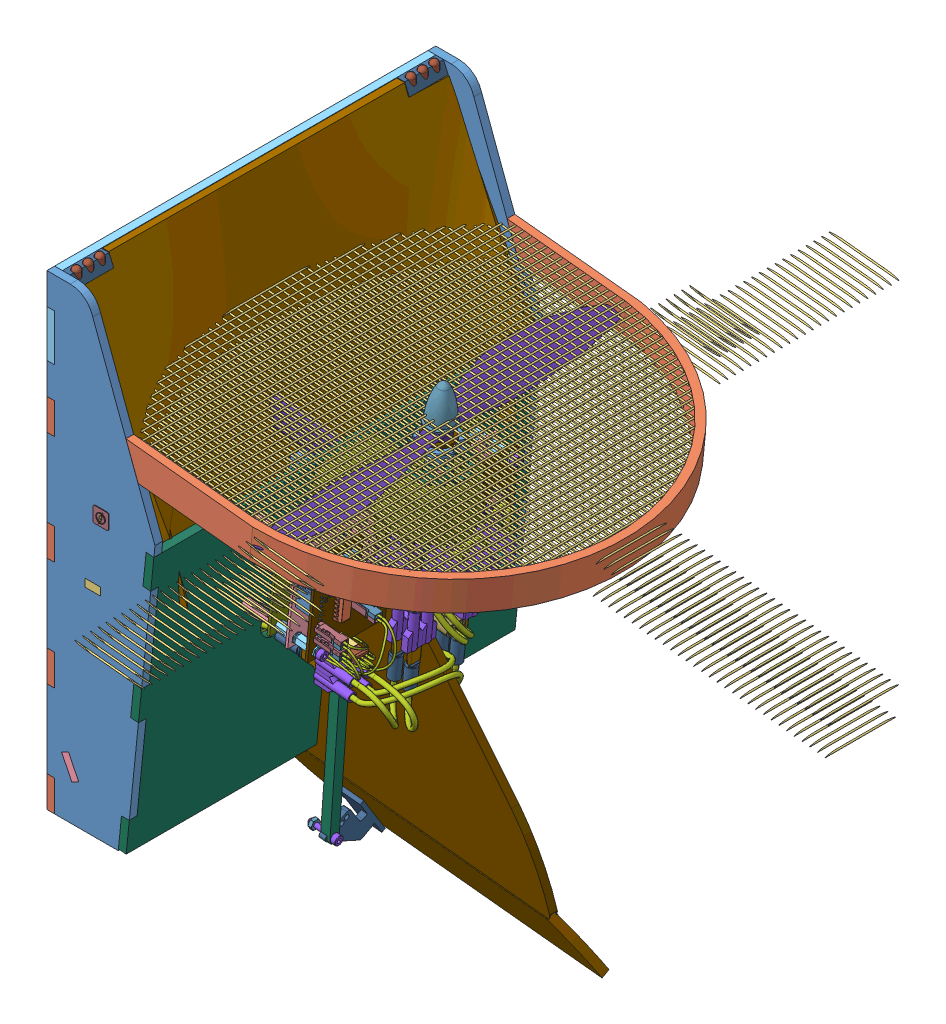
SolidWorks assembly AssTotaleSimu, configuration Défaut. Lengths in mm. (continued)
Components (placement in the parent): (continued)
- AssStructSimu-1: AssStructSimu [Défaut] at (-125.7658 -1.8483 624.6548) x (1 0 0) z (0 0 -1) size (323.53 326.04 251.6) (continued)
  - AssCarte-1: AssCarte [Défaut] at (-42.8534 32.2132 302.028) x (-0.101852 0.9948 0) z (0.9948 0.101852 0) size (91.19 130.57 98.45) (continued)
    - carte_onduleur_v4-1: carte_onduleur_v4 [Défaut] at (-25.7639 0.8332 112.9379) size (66.52 130.57 82.34) (continued)
      - CARTE_CMD-1: CARTE_CMD [Défaut] at (25 57.2 0.803) size (60.1 130 26.71) (continued)
        - Open CASCADE STEP translator 6.8 1.20.1-1: Open CASCADE STEP translator 6.8 1.20.1 [Défaut] at origin size (60.1 130 26.71) (continued)
          - Body_1_4-1: Body_1_4 [Défaut] at (-55 5 12) size (60.1 130 26.71) (continued)
            - 40_2-1: 40_2 [Défaut] at (26.2 -12.2 0.803) x (0 -1 0) z (0 0 1) size (2.34 1.04 0.5) (continued)
              - =_[0_1_1_30]-1: =_[0_1_1_30] [Défaut] at origin size (2.34 1.04 0.5) (continued)
                - 33_2-1: 33_2 [Défaut] at (0.3048 0 0) x (-1 0 0) z (0 0 1) size (0.51 1.02 0.5)
                - 34-1: 34 [Défaut] at origin size (0.51 1.02 0.5)
            - 42_2-1: 42_2 [Défaut] at (24.4 -119.2 0.803) size (2.34 1.04 0.5)
              - =_[0_1_1_30]-1: =_[0_1_1_30] [Défaut] at origin size (2.34 1.04 0.5)
                - 32_2-1: 32_2 [Défaut] at origin size (2.29 1.04 0.43)
                - 33_2-1: 33_2 [Défaut] at (0.3048 0 0) x (-1 0 0) z (0 0 1) size (0.51 1.02 0.5)
                - 34-1: 34 [Défaut] at origin size (0.51 1.02 0.5)
            - 45-1: 45 [Défaut] at (46.4 -125 0.803) size (5.08 5 14.3)
              - =_[0_1_1_38]-1: =_[0_1_1_38] [Défaut] at origin size (5.08 5 14.3)
                - 190-1: 190 [Défaut] at (1.2 0 11) size (5.08 5 14.3)
            - 48-1: 48 [Défaut] at (40.1 -125 0.803) size (5.08 5 14.3)
              - =_[0_1_1_41]-1: =_[0_1_1_41] [Défaut] at origin size (5.08 5 14.3)
                - 190-1: 190 [Défaut] at (1.2 0 11) size (5.08 5 14.3)
            - 51-1: 51 [Défaut] at (6.4 -119.9 0.803) x (0 1 0) z (0 0 1) size (15.24 2.54 7.37)
              - =_[0_1_1_43]-1: =_[0_1_1_43] [Défaut] at origin size (15.24 2.54 7.37)
                - 49_2-1: 49_2 [Défaut] at (6.5 0 0) x (1 0 0) z (0 -1 0) size (15.24 7.37 2.54)
            - 57_2-1: 57_2 [Défaut] at (50.8796 -121.1 -0.803) x (-1 0 0) z (0 0 -1) size (2.54 1.98 0.64)
              - =_[0_1_1_46]-1: =_[0_1_1_46] [Défaut] at origin size (2.54 1.98 0.64)
                - 52-1: 52 [Défaut] at origin size (2.54 1.14 0.58)
                - 53-1: 53 [Défaut] x (0 -1 0) z (0 0 1) size (0.43 0.51 0.38)
                - 54-1: 54 [Défaut] at (1.8796 1.8796 0) x (0 -1 0) z (0 0 1) size (0.43 0.51 0.38)
                - 55-1: 55 [Défaut] at (-0.9652 -2.8448 0) x (0 1 0) z (0 0 1) size (0.41 0.51 0.38)
            - 59_2-1: 59_2 [Défaut] at (43.6398 -120.995 -0.803) x (-1 0 0) z (0 0 -1) size (2.54 1.98 0.64)
              - =_[0_1_1_46]-1: =_[0_1_1_46] [Défaut] at origin size (2.54 1.98 0.64)
                - 52-1: 52 [Défaut] at origin size (2.54 1.14 0.58)
                - 53-1: 53 [Défaut] x (0 -1 0) z (0 0 1) size (0.43 0.51 0.38)
                - 54-1: 54 [Défaut] at (1.8796 1.8796 0) x (0 -1 0) z (0 0 1) size (0.43 0.51 0.38)
                - 55-1: 55 [Défaut] at (-0.9652 -2.8448 0) x (0 1 0) z (0 0 1) size (0.41 0.51 0.38)
            - 61_2-1: 61_2 [Défaut] at (47.6 -119.9 -0.803) x (-1 0 0) z (0 0 -1) size (2.34 1.04 0.5)
              - =_[0_1_1_30]-1: =_[0_1_1_30] [Défaut] at origin size (2.34 1.04 0.5)
                - 32_2-1: 32_2 [Défaut] at origin size (2.29 1.04 0.43)
                - 33_2-1: 33_2 [Défaut] at (0.3048 0 0) x (-1 0 0) z (0 0 1) size (0.51 1.02 0.5)
                - 34-1: 34 [Défaut] at origin size (0.51 1.02 0.5)
            - 63-1: 63 [Défaut] at (40.4 -119.9 -0.803) x (-1 0 0) z (0 0 -1) size (2.34 1.04 0.5)
              - =_[0_1_1_30]-1: =_[0_1_1_30] [Défaut] at origin size (2.34 1.04 0.5)
                - 32_2-1: 32_2 [Défaut] at origin size (2.29 1.04 0.43)
                - 33_2-1: 33_2 [Défaut] at (0.3048 0 0) x (-1 0 0) z (0 0 1) size (0.51 1.02 0.5)
                - 34-1: 34 [Défaut] at origin size (0.51 1.02 0.5)
            - 68-1: 68 [Défaut] at (47.7 -21.8 -0.803) x (0 1 0) z (0 0 -1) size (2.34 1.04 0.5)
              - =_[0_1_1_55]-1: =_[0_1_1_55] [Défaut] at origin size (2.34 1.04 0.5)
                - 64-1: 64 [Défaut] at origin size (2.29 1.04 0.43)
                - 65-1: 65 [Défaut] at (0.3048 0 0) x (-1 0 0) z (0 0 1) size (0.51 1.02 0.5)
                - 66-1: 66 [Défaut] at origin size (0.51 1.02 0.5)
            - 70-1: 70 [Défaut] at (47.6 -121.7 -0.803) x (-1 0 0) z (0 0 -1) size (2.34 1.04 0.5)
              - =_[0_1_1_30]-1: =_[0_1_1_30] [Défaut] at origin size (2.34 1.04 0.5)
                - 32_2-1: 32_2 [Défaut] at origin size (2.29 1.04 0.43)
                - 33_2-1: 33_2 [Défaut] at (0.3048 0 0) x (-1 0 0) z (0 0 1) size (0.51 1.02 0.5)
                - 34-1: 34 [Défaut] at origin size (0.51 1.02 0.5)
            - 72-1: 72 [Défaut] at (40.4 -121.5 -0.803) x (-1 0 0) z (0 0 -1) size (2.34 1.04 0.5)
              - =_[0_1_1_30]-1: =_[0_1_1_30] [Défaut] at origin size (2.34 1.04 0.5)
                - 32_2-1: 32_2 [Défaut] at origin size (2.29 1.04 0.43)
                - 33_2-1: 33_2 [Défaut] at (0.3048 0 0) x (-1 0 0) z (0 0 1) size (0.51 1.02 0.5)
                - 34-1: 34 [Défaut] at origin size (0.51 1.02 0.5)
            - 74-1: 74 [Défaut] at (47.7 -18.3 -0.803) x (0 1 0) z (0 0 -1) size (2.34 1.04 0.5)
              - =_[0_1_1_55]-1: =_[0_1_1_55] [Défaut] at origin size (2.34 1.04 0.5)
                - 64-1: 64 [Défaut] at origin size (2.29 1.04 0.43)
                - 65-1: 65 [Défaut] at (0.3048 0 0) x (-1 0 0) z (0 0 1) size (0.51 1.02 0.5)
                - 66-1: 66 [Défaut] at origin size (0.51 1.02 0.5)
            - 76-1: 76 [Défaut] at (45.5 -118.3 -0.803) x (1 0 0) z (0 0 -1) size (2.34 1.04 0.5)
              - =_[0_1_1_30]-1: =_[0_1_1_30] [Défaut] at origin size (2.34 1.04 0.5)
                - 32_2-1: 32_2 [Défaut] at origin size (2.29 1.04 0.43)
                - 33_2-1: 33_2 [Défaut] at (0.3048 0 0) x (-1 0 0) z (0 0 1) size (0.51 1.02 0.5)
                - 34-1: 34 [Défaut] at origin size (0.51 1.02 0.5)
            - 78-1: 78 [Défaut] at (38.2 -118.3 -0.803) x (1 0 0) z (0 0 -1) size (2.34 1.04 0.5)
              - =_[0_1_1_30]-1: =_[0_1_1_30] [Défaut] at origin size (2.34 1.04 0.5)
                - 32_2-1: 32_2 [Défaut] at origin size (2.29 1.04 0.43)
                - 33_2-1: 33_2 [Défaut] at (0.3048 0 0) x (-1 0 0) z (0 0 1) size (0.51 1.02 0.5)
                - 34-1: 34 [Défaut] at origin size (0.51 1.02 0.5)
            - 80-1: 80 [Défaut] at (28.6 -10.7 0.803) x (0 1 0) z (0 0 1) size (2.34 1.04 0.5)
              - =_[0_1_1_55]-1: =_[0_1_1_55] [Défaut] at origin size (2.34 1.04 0.5)
                - 64-1: 64 [Défaut] at origin size (2.29 1.04 0.43)
                - 65-1: 65 [Défaut] at (0.3048 0 0) x (-1 0 0) z (0 0 1) size (0.51 1.02 0.5)
                - 66-1: 66 [Défaut] at origin size (0.51 1.02 0.5)
            - 82-1: 82 [Défaut] at (23.7 -10.7 0.803) x (0 1 0) z (0 0 1) size (2.34 1.04 0.5)
              - =_[0_1_1_55]-1: =_[0_1_1_55] [Défaut] at origin size (2.34 1.04 0.5)
                - 64-1: 64 [Défaut] at origin size (2.29 1.04 0.43)
                - 65-1: 65 [Défaut] at (0.3048 0 0) x (-1 0 0) z (0 0 1) size (0.51 1.02 0.5)
                - 66-1: 66 [Défaut] at origin size (0.51 1.02 0.5)
            - 84-1: 84 [Défaut] at (26.2 -10.7 0.803) x (0 1 0) z (0 0 1) size (2.34 1.04 0.5)
              - =_[0_1_1_55]-1: =_[0_1_1_55] [Défaut] at origin size (2.34 1.04 0.5)
                - 64-1: 64 [Défaut] at origin size (2.29 1.04 0.43)
                - 65-1: 65 [Défaut] at (0.3048 0 0) x (-1 0 0) z (0 0 1) size (0.51 1.02 0.5)
                - 66-1: 66 [Défaut] at origin size (0.51 1.02 0.5)
            - 86-1: 86 [Défaut] at (23.0336 -119.2 0.803) x (-1 0 0) z (0 0 1) size (2.34 1.04 0.5)
              - =_[0_1_1_55]-1: =_[0_1_1_55] [Défaut] at origin size (2.34 1.04 0.5)
                - 64-1: 64 [Défaut] at origin size (2.29 1.04 0.43)
                - 65-1: 65 [Défaut] at (0.3048 0 0) x (-1 0 0) z (0 0 1) size (0.51 1.02 0.5)
                - 66-1: 66 [Défaut] at origin size (0.51 1.02 0.5)
            - 88-1: 88 [Défaut] at (14.1 -114.2 0.803) x (0 -1 0) z (0 0 1) size (2.34 1.04 0.5)
              - =_[0_1_1_55]-1: =_[0_1_1_55] [Défaut] at origin size (2.34 1.04 0.5)
                - 64-1: 64 [Défaut] at origin size (2.29 1.04 0.43)
                - 65-1: 65 [Défaut] at (0.3048 0 0) x (-1 0 0) z (0 0 1) size (0.51 1.02 0.5)
                - 66-1: 66 [Défaut] at origin size (0.51 1.02 0.5)
            - 90-1: 90 [Défaut] at (43.6 -107.8 -0.803) x (1 0 0) z (0 0 -1) size (2.34 1.04 0.5)
              - =_[0_1_1_55]-1: =_[0_1_1_55] [Défaut] at origin size (2.34 1.04 0.5)
                - 64-1: 64 [Défaut] at origin size (2.29 1.04 0.43)
                - 65-1: 65 [Défaut] at (0.3048 0 0) x (-1 0 0) z (0 0 1) size (0.51 1.02 0.5)
                - 66-1: 66 [Défaut] at origin size (0.51 1.02 0.5)
            - 92-1: 92 [Défaut] at (43.6 -106 -0.803) x (1 0 0) z (0 0 -1) size (2.34 1.04 0.5)
              - =_[0_1_1_55]-1: =_[0_1_1_55] [Défaut] at origin size (2.34 1.04 0.5)
                - 64-1: 64 [Défaut] at origin size (2.29 1.04 0.43)
                - 65-1: 65 [Défaut] at (0.3048 0 0) x (-1 0 0) z (0 0 1) size (0.51 1.02 0.5)
                - 66-1: 66 [Défaut] at origin size (0.51 1.02 0.5)
            - 175-1: 175 [Défaut] at (10 -21.7 0.803) x (0 -1 0) z (0 0 1) size (15 25.4 12.78)
              - =_[0_1_1_72]-1: =_[0_1_1_72] [Défaut] at origin size (15 25.4 12.78)
                - 173-1: 173 [Défaut] at (-1.4 -1 12) x (-1 0 0) z (0 1 0) size (15 12.78 25.4)
                  - board_1-1: board_1 [Défaut] at (-7.5 -1.57 12.5) size (15 1.57 25)
                  - hole_plating_20-1: hole_plating_20 [Défaut] at (-1.5 0 23.93) size (1.5 0.01 1.5)
                  - hole_plating_20-2: hole_plating_20 [Défaut] at (-1.5 0 21.39) size (1.5 0.01 1.5)
                  - hole_plating_20-3: hole_plating_20 [Défaut] at (-1.5 0 8.69) size (1.5 0.01 1.5)
                  - hole_plating_20-4: hole_plating_20 [Défaut] at (-1.5 -1.58 13.77) size (1.5 0.01 1.5)
                  - hole_plating_20-5: hole_plating_20 [Défaut] at (-1.5 0 16.31) size (1.5 0.01 1.5)
                  - hole_plating_20-6: hole_plating_20 [Défaut] at (-1.5 0 18.85) size (1.5 0.01 1.5)
                  - hole_plating_20-7: hole_plating_20 [Défaut] at (-1.5 0 13.77) size (1.5 0.01 1.5)
                  - hole_plating_20-8: hole_plating_20 [Défaut] at (-1.5 -1.58 11.23) size (1.5 0.01 1.5)
                  - hole_plating_20-9: hole_plating_20 [Défaut] at (-1.5 -1.58 18.85) size (1.5 0.01 1.5)
                  - hole_plating_20-10: hole_plating_20 [Défaut] at (-1.5 -1.58 6.15) size (1.5 0.01 1.5)
                  - hole_plating_20-11: hole_plating_20 [Défaut] at (-1.5 0 1.07) size (1.5 0.01 1.5)
                  - hole_plating_20-12: hole_plating_20 [Défaut] at (-1.5 -1.58 3.61) size (1.5 0.01 1.5)
                  - hole_plating_20-13: hole_plating_20 [Défaut] at (-1.5 -1.58 1.07) size (1.5 0.01 1.5)
                  - hole_plating_20-14: hole_plating_20 [Défaut] at (-1.5 -1.58 8.69) size (1.5 0.01 1.5)
                  - hole_plating_20-15: hole_plating_20 [Défaut] at (-1.5 -1.58 16.31) size (1.5 0.01 1.5)
                  - hole_plating_20-16: hole_plating_20 [Défaut] at (-1.5 0 11.23) size (1.5 0.01 1.5)
                  - hole_plating_20-17: hole_plating_20 [Défaut] at (-1.5 0 3.61) size (1.5 0.01 1.5)
                  - hole_plating_20-18: hole_plating_20 [Défaut] at (-1.5 -1.58 21.39) size (1.5 0.01 1.5)
                  - hole_plating_20-19: hole_plating_20 [Défaut] at (-1.5 0 6.15) size (1.5 0.01 1.5)
                  - hole_plating_20-20: hole_plating_20 [Défaut] at (-1.5 -1.58 23.93) size (1.5 0.01 1.5)
                  - Pin_Header_1x10_TH_Pitch_2.54mm_1-1: Pin_Header_1x10_TH_Pitch_2.54mm_1 [Défaut] at (-1.5 -1.5786 23.93) x (0 0 -1) z (0 -1 0) size (25.4 2.54 12.7)
                    - 124-1: 124 [Défaut] at origin size (25.4 2.54 2.8)
                      - =_[0_1_1_77]-1: =_[0_1_1_77] [Défaut] at origin size (2.54 2.54 2.8)
                      - =_[0_1_1_79]-1: =_[0_1_1_79] [Défaut] at origin size (2.54 2.54 2.8)
                      - =_[0_1_1_80]-1: =_[0_1_1_80] [Défaut] at origin size (2.54 2.54 2.8)
                      - =_[0_1_1_81]-1: =_[0_1_1_81] [Défaut] at origin size (2.54 2.54 2.8)
                      - =_[0_1_1_82]-1: =_[0_1_1_82] [Défaut] at origin size (2.54 2.54 2.8)
                      - =_[0_1_1_83]-1: =_[0_1_1_83] [Défaut] at origin size (2.54 2.54 2.8)
                      - =_[0_1_1_84]-1: =_[0_1_1_84] [Défaut] at origin size (2.54 2.54 2.8)
                      - =_[0_1_1_85]-1: =_[0_1_1_85] [Défaut] at origin size (2.54 2.54 2.8)
                      - =_[0_1_1_86]-1: =_[0_1_1_86] [Défaut] at origin size (2.54 2.54 2.8)
                      - =_[0_1_1_87]-1: =_[0_1_1_87] [Défaut] at origin size (2.54 2.54 2.8)
                    - 135-1: 135 [Défaut] at origin size (23.49 0.63 12.7)
                      - =_[0_1_1_88]-1: =_[0_1_1_88] [Défaut] at origin size (0.63 0.63 12.7)
                      - =_[0_1_1_90]-1: =_[0_1_1_90] [Défaut] at origin size (0.63 0.63 12.7)
                      - =_[0_1_1_91]-1: =_[0_1_1_91] [Défaut] at origin size (0.63 0.63 12.7)
                      - =_[0_1_1_92]-1: =_[0_1_1_92] [Défaut] at origin size (0.63 0.63 12.7)
                      - =_[0_1_1_93]-1: =_[0_1_1_93] [Défaut] at origin size (0.63 0.63 12.7)
                      - =_[0_1_1_94]-1: =_[0_1_1_94] [Défaut] at origin size (0.63 0.63 12.7)
                      - =_[0_1_1_95]-1: =_[0_1_1_95] [Défaut] at origin size (0.63 0.63 12.7)
                      - =_[0_1_1_96]-1: =_[0_1_1_96] [Défaut] at origin size (0.63 0.63 12.7)
                      - =_[0_1_1_97]-1: =_[0_1_1_97] [Défaut] at origin size (0.63 0.63 12.7)
                      - =_[0_1_1_98]-1: =_[0_1_1_98] [Défaut] at origin size (0.63 0.63 12.7)
                  - MPU-9250_1-1: MPU-9250_1 [Défaut] at (-8 0.05 12.5) x (-1 0 0) z (0 1 0) size (3 3 1.05)
                  - tantalum_10uF_1-1: tantalum_10uF_1 [Défaut] at (-13.167 0.1 10.9372) x (0 0 1) z (0 1 0) size (3.4 1.6 1.71)
                  - SOT23_5_1-1: SOT23_5_1 [Défaut] at (-7.475 -0.0136 21) x (0 0 1) z (0 1 0) size (3 3.2 0.92)
                  - RESC-0603_5-1: RESC-0603_5 [Défaut] at (-6.85 0 7.45) x (1 0 0) z (0 1 0) size (1.7 0.9 0.55)
                    - 143-1: 143 [Défaut] at origin size (1.7 0.9 0.55)
                      - =_[0_1_1_103]-1: =_[0_1_1_103] [Défaut] at origin size (0.4 0.9 0.53)
                      - =_[0_1_1_105]-1: =_[0_1_1_105] [Défaut] at origin size (0.4 0.9 0.53)
                      - =_[0_1_1_106]-1: =_[0_1_1_106] [Défaut] at origin size (1.64 0.9 0.52)
                    - 152-1: 152 [Défaut] at origin
                      - =_[0_1_1_107]-1: =_[0_1_1_107] [Défaut] at origin
                      - =_[0_1_1_109]-1: =_[0_1_1_109] [Défaut] at origin
                      - =_[0_1_1_110]-1: =_[0_1_1_110] [Défaut] at origin
                      - =_[0_1_1_111]-1: =_[0_1_1_111] [Défaut] at origin
                      - =_[0_1_1_112]-1: =_[0_1_1_112] [Défaut] at origin
                      - =_[0_1_1_113]-1: =_[0_1_1_113] [Défaut] at origin
                      - =_[0_1_1_114]-1: =_[0_1_1_114] [Défaut] at origin
                      - =_[0_1_1_115]-1: =_[0_1_1_115] [Défaut] at origin
                  - RESC-0603_5-2: RESC-0603_5 [Défaut] at (-9.85 0 16.05) x (1 0 0) z (0 1 0) size (1.7 0.9 0.55)
                    - 143-1: 143 [Défaut] at origin size (1.7 0.9 0.55)
                      - =_[0_1_1_103]-1: =_[0_1_1_103] [Défaut] at origin size (0.4 0.9 0.53)
                      - =_[0_1_1_105]-1: =_[0_1_1_105] [Défaut] at origin size (0.4 0.9 0.53)
                      - =_[0_1_1_106]-1: =_[0_1_1_106] [Défaut] at origin size (1.64 0.9 0.52)
                    - 152-1: 152 [Défaut] at origin
                      - =_[0_1_1_107]-1: =_[0_1_1_107] [Défaut] at origin
                      - =_[0_1_1_109]-1: =_[0_1_1_109] [Défaut] at origin
                      - =_[0_1_1_110]-1: =_[0_1_1_110] [Défaut] at origin
                      - =_[0_1_1_111]-1: =_[0_1_1_111] [Défaut] at origin
                      - =_[0_1_1_112]-1: =_[0_1_1_112] [Défaut] at origin
                      - =_[0_1_1_113]-1: =_[0_1_1_113] [Défaut] at origin
                      - =_[0_1_1_114]-1: =_[0_1_1_114] [Défaut] at origin
                      - =_[0_1_1_115]-1: =_[0_1_1_115] [Défaut] at origin
                  - RESC-0603_5-3: RESC-0603_5 [Défaut] at (-6.85 0 17.55) x (1 0 0) z (0 1 0) size (1.7 0.9 0.55)
                    - 143-1: 143 [Défaut] at origin size (1.7 0.9 0.55)
                      - =_[0_1_1_103]-1: =_[0_1_1_103] [Défaut] at origin size (0.4 0.9 0.53)
                      - =_[0_1_1_105]-1: =_[0_1_1_105] [Défaut] at origin size (0.4 0.9 0.53)
                      - =_[0_1_1_106]-1: =_[0_1_1_106] [Défaut] at origin size (1.64 0.9 0.52)
                    - 152-1: 152 [Défaut] at origin
                      - =_[0_1_1_107]-1: =_[0_1_1_107] [Défaut] at origin
                      - =_[0_1_1_109]-1: =_[0_1_1_109] [Défaut] at origin
                      - =_[0_1_1_110]-1: =_[0_1_1_110] [Défaut] at origin
                      - =_[0_1_1_111]-1: =_[0_1_1_111] [Défaut] at origin
                      - =_[0_1_1_112]-1: =_[0_1_1_112] [Défaut] at origin
                      - =_[0_1_1_113]-1: =_[0_1_1_113] [Défaut] at origin
                      - =_[0_1_1_114]-1: =_[0_1_1_114] [Défaut] at origin
                      - =_[0_1_1_115]-1: =_[0_1_1_115] [Défaut] at origin
                  - RESC-0603_5-4: RESC-0603_5 [Défaut] at (-6.85 0 16.05) x (1 0 0) z (0 1 0) size (1.7 0.9 0.55)
                    - 143-1: 143 [Défaut] at origin size (1.7 0.9 0.55)
                      - =_[0_1_1_103]-1: =_[0_1_1_103] [Défaut] at origin size (0.4 0.9 0.53)
                      - =_[0_1_1_105]-1: =_[0_1_1_105] [Défaut] at origin size (0.4 0.9 0.53)
                      - =_[0_1_1_106]-1: =_[0_1_1_106] [Défaut] at origin size (1.64 0.9 0.52)
                    - 152-1: 152 [Défaut] at origin
                      - =_[0_1_1_107]-1: =_[0_1_1_107] [Défaut] at origin
                      - =_[0_1_1_109]-1: =_[0_1_1_109] [Défaut] at origin
                      - =_[0_1_1_110]-1: =_[0_1_1_110] [Défaut] at origin
                      - =_[0_1_1_111]-1: =_[0_1_1_111] [Défaut] at origin
                      - =_[0_1_1_112]-1: =_[0_1_1_112] [Défaut] at origin
                      - =_[0_1_1_113]-1: =_[0_1_1_113] [Défaut] at origin
                      - =_[0_1_1_114]-1: =_[0_1_1_114] [Défaut] at origin
                      - =_[0_1_1_115]-1: =_[0_1_1_115] [Défaut] at origin
                  - RESC-0603_5-5: RESC-0603_5 [Défaut] at (-6.85 0 5.95) x (1 0 0) z (0 1 0) size (1.7 0.9 0.55)
                    - 143-1: 143 [Défaut] at origin size (1.7 0.9 0.55)
                      - =_[0_1_1_103]-1: =_[0_1_1_103] [Défaut] at origin size (0.4 0.9 0.53)
                      - =_[0_1_1_105]-1: =_[0_1_1_105] [Défaut] at origin size (0.4 0.9 0.53)
                      - =_[0_1_1_106]-1: =_[0_1_1_106] [Défaut] at origin size (1.64 0.9 0.52)
                    - 152-1: 152 [Défaut] at origin
                      - =_[0_1_1_107]-1: =_[0_1_1_107] [Défaut] at origin
                      - =_[0_1_1_109]-1: =_[0_1_1_109] [Défaut] at origin
                      - =_[0_1_1_110]-1: =_[0_1_1_110] [Défaut] at origin
                      - =_[0_1_1_111]-1: =_[0_1_1_111] [Défaut] at origin
                      - =_[0_1_1_112]-1: =_[0_1_1_112] [Défaut] at origin
                      - =_[0_1_1_113]-1: =_[0_1_1_113] [Défaut] at origin
                      - =_[0_1_1_114]-1: =_[0_1_1_114] [Défaut] at origin
                      - =_[0_1_1_115]-1: =_[0_1_1_115] [Défaut] at origin
                  - CAPC-0603-T0.9-BN_5-1: CAPC-0603-T0.9-BN_5 [Défaut] at (-9.85 0 8.95) x (1 0 0) z (0 1 0) size (1.7 0.9 0.9)
                    - =_[0_1_1_117]-1: =_[0_1_1_117] [Défaut] at origin size (1.7 0.9 0.9)
                    - 167-1: 167 [Défaut] at origin
                      - =_[0_1_1_118]-1: =_[0_1_1_118] [Défaut] at origin
                      - =_[0_1_1_120]-1: =_[0_1_1_120] [Défaut] at origin
                      - =_[0_1_1_121]-1: =_[0_1_1_121] [Défaut] at origin
                      - =_[0_1_1_122]-1: =_[0_1_1_122] [Défaut] at origin
                      - =_[0_1_1_123]-1: =_[0_1_1_123] [Défaut] at origin
                      - =_[0_1_1_124]-1: =_[0_1_1_124] [Défaut] at origin
                      - =_[0_1_1_125]-1: =_[0_1_1_125] [Défaut] at origin
                      - =_[0_1_1_126]-1: =_[0_1_1_126] [Défaut] at origin
                  - CAPC-0603-T0.9-BN_5-2: CAPC-0603-T0.9-BN_5 [Défaut] at (-6.85 0 8.95) x (1 0 0) z (0 1 0) size (1.7 0.9 0.9)
                    - =_[0_1_1_117]-1: =_[0_1_1_117] [Défaut] at origin size (1.7 0.9 0.9)
                    - 167-1: 167 [Défaut] at origin
                      - =_[0_1_1_118]-1: =_[0_1_1_118] [Défaut] at origin
                      - =_[0_1_1_120]-1: =_[0_1_1_120] [Défaut] at origin
                      - =_[0_1_1_121]-1: =_[0_1_1_121] [Défaut] at origin
                      - =_[0_1_1_122]-1: =_[0_1_1_122] [Défaut] at origin
                      - =_[0_1_1_123]-1: =_[0_1_1_123] [Défaut] at origin
                      - =_[0_1_1_124]-1: =_[0_1_1_124] [Défaut] at origin
                      - =_[0_1_1_125]-1: =_[0_1_1_125] [Défaut] at origin
                      - =_[0_1_1_126]-1: =_[0_1_1_126] [Défaut] at origin
                  - CAPC-0603-T0.9-BN_5-3: CAPC-0603-T0.9-BN_5 [Défaut] at (-6.85 0 19.05) x (1 0 0) z (0 1 0) size (1.7 0.9 0.9)
                    - =_[0_1_1_117]-1: =_[0_1_1_117] [Défaut] at origin size (1.7 0.9 0.9)
                    - 167-1: 167 [Défaut] at origin
                      - =_[0_1_1_118]-1: =_[0_1_1_118] [Défaut] at origin
                      - =_[0_1_1_120]-1: =_[0_1_1_120] [Défaut] at origin
                      - =_[0_1_1_121]-1: =_[0_1_1_121] [Défaut] at origin
                      - =_[0_1_1_122]-1: =_[0_1_1_122] [Défaut] at origin
                      - =_[0_1_1_123]-1: =_[0_1_1_123] [Défaut] at origin
                      - =_[0_1_1_124]-1: =_[0_1_1_124] [Défaut] at origin
                      - =_[0_1_1_125]-1: =_[0_1_1_125] [Défaut] at origin
                      - =_[0_1_1_126]-1: =_[0_1_1_126] [Défaut] at origin
                  - CAPC-0603-T0.9-BN_5-4: CAPC-0603-T0.9-BN_5 [Défaut] at (-9.85 0 7.45) x (1 0 0) z (0 1 0) size (1.7 0.9 0.9)
                    - =_[0_1_1_117]-1: =_[0_1_1_117] [Défaut] at origin size (1.7 0.9 0.9)
                    - 167-1: 167 [Défaut] at origin
                      - =_[0_1_1_118]-1: =_[0_1_1_118] [Défaut] at origin
                      - =_[0_1_1_120]-1: =_[0_1_1_120] [Défaut] at origin
                      - =_[0_1_1_121]-1: =_[0_1_1_121] [Défaut] at origin
                      - =_[0_1_1_122]-1: =_[0_1_1_122] [Défaut] at origin
                      - =_[0_1_1_123]-1: =_[0_1_1_123] [Défaut] at origin
                      - =_[0_1_1_124]-1: =_[0_1_1_124] [Défaut] at origin
                      - =_[0_1_1_125]-1: =_[0_1_1_125] [Défaut] at origin
                      - =_[0_1_1_126]-1: =_[0_1_1_126] [Défaut] at origin
                  - CAPC-0603-T0.9-BN_5-5: CAPC-0603-T0.9-BN_5 [Défaut] at (-9.85 0 17.55) x (1 0 0) z (0 1 0) size (1.7 0.9 0.9)
                    - =_[0_1_1_117]-1: =_[0_1_1_117] [Défaut] at origin size (1.7 0.9 0.9)
                    - 167-1: 167 [Défaut] at origin
                      - =_[0_1_1_118]-1: =_[0_1_1_118] [Défaut] at origin
                      - =_[0_1_1_120]-1: =_[0_1_1_120] [Défaut] at origin
                      - =_[0_1_1_121]-1: =_[0_1_1_121] [Défaut] at origin
                      - =_[0_1_1_122]-1: =_[0_1_1_122] [Défaut] at origin
                      - =_[0_1_1_123]-1: =_[0_1_1_123] [Défaut] at origin
                      - =_[0_1_1_124]-1: =_[0_1_1_124] [Défaut] at origin
                      - =_[0_1_1_125]-1: =_[0_1_1_125] [Défaut] at origin
                      - =_[0_1_1_126]-1: =_[0_1_1_126] [Défaut] at origin
            - 177-1: 177 [Défaut] at (52.1 -16.5 -0.803) x (1 0 0) z (0 0 -1) size (2.34 1.04 0.5)
              - =_[0_1_1_30]-1: =_[0_1_1_30] [Défaut] at origin size (2.34 1.04 0.5)
                - 32_2-1: 32_2 [Défaut] at origin size (2.29 1.04 0.43)
                - 33_2-1: 33_2 [Défaut] at (0.3048 0 0) x (-1 0 0) z (0 0 1) size (0.51 1.02 0.5)
                - 34-1: 34 [Défaut] at origin size (0.51 1.02 0.5)
            - 179-1: 179 [Défaut] at (22.5336 -121.5 -0.803) x (-1 0 0) z (0 0 -1) size (2.34 1.04 0.5)
              - =_[0_1_1_30]-1: =_[0_1_1_30] [Défaut] at origin size (2.34 1.04 0.5)
                - 32_2-1: 32_2 [Défaut] at origin size (2.29 1.04 0.43)
                - 33_2-1: 33_2 [Défaut] at (0.3048 0 0) x (-1 0 0) z (0 0 1) size (0.51 1.02 0.5)
                - 34-1: 34 [Défaut] at origin size (0.51 1.02 0.5)
            - 181-1: 181 [Défaut] at (48.6 -127 -0.803) x (-1 0 0) z (0 0 -1) size (2.34 1.04 0.5)
              - =_[0_1_1_30]-1: =_[0_1_1_30] [Défaut] at origin size (2.34 1.04 0.5)
                - 32_2-1: 32_2 [Défaut] at origin size (2.29 1.04 0.43)
                - 33_2-1: 33_2 [Défaut] at (0.3048 0 0) x (-1 0 0) z (0 0 1) size (0.51 1.02 0.5)
                - 34-1: 34 [Défaut] at origin size (0.51 1.02 0.5)
            - 183-1: 183 [Défaut] at (26.0189 -121.5 0.803) size (2.34 1.04 0.5)
              - =_[0_1_1_30]-1: =_[0_1_1_30] [Défaut] at origin size (2.34 1.04 0.5)
                - 32_2-1: 32_2 [Défaut] at origin size (2.29 1.04 0.43)
                - 33_2-1: 33_2 [Défaut] at (0.3048 0 0) x (-1 0 0) z (0 0 1) size (0.51 1.02 0.5)
                - 34-1: 34 [Défaut] at origin size (0.51 1.02 0.5)
            - 185-1: 185 [Défaut] at (30.3664 -19 -0.803) x (1 0 0) z (0 0 -1) size (2.34 1.04 0.5)
              - =_[0_1_1_30]-1: =_[0_1_1_30] [Défaut] at origin size (2.34 1.04 0.5)
                - 32_2-1: 32_2 [Défaut] at origin size (2.29 1.04 0.43)
                - 33_2-1: 33_2 [Défaut] at (0.3048 0 0) x (-1 0 0) z (0 0 1) size (0.51 1.02 0.5)
                - 34-1: 34 [Défaut] at origin size (0.51 1.02 0.5)
            - 187-1: 187 [Défaut] at (51.7 -114.3 -0.803) x (0 1 0) z (0 0 -1) size (2.34 1.04 0.5)
              - =_[0_1_1_30]-1: =_[0_1_1_30] [Défaut] at origin size (2.34 1.04 0.5)
                - 32_2-1: 32_2 [Défaut] at origin size (2.29 1.04 0.43)
                - 33_2-1: 33_2 [Défaut] at (0.3048 0 0) x (-1 0 0) z (0 0 1) size (0.51 1.02 0.5)
                - 34-1: 34 [Défaut] at origin size (0.51 1.02 0.5)
            - 189-1: 189 [Défaut] at (50 -114.3 -0.803) x (0 1 0) z (0 0 -1) size (2.34 1.04 0.5)
              - =_[0_1_1_30]-1: =_[0_1_1_30] [Défaut] at origin size (2.34 1.04 0.5)
                - 32_2-1: 32_2 [Défaut] at origin size (2.29 1.04 0.43)
                - 33_2-1: 33_2 [Défaut] at (0.3048 0 0) x (-1 0 0) z (0 0 1) size (0.51 1.02 0.5)
                - 34-1: 34 [Défaut] at origin size (0.51 1.02 0.5)
            - 192-1: 192 [Défaut] at (37.94 -103.3308 0.803) x (-1 0 0) z (0 0 1) size (5.08 5 14.3)
              - =_[0_1_1_135]-1: =_[0_1_1_135] [Défaut] at origin size (5.08 5 14.3)
                - 190-1: 190 [Défaut] at (1.2 0 11) size (5.08 5 14.3)
            - 194-1: 194 [Défaut] at (32.7796 -102.6 -0.803) x (-1 0 0) z (0 0 -1) size (2.54 1.98 0.64)
              - =_[0_1_1_46]-1: =_[0_1_1_46] [Défaut] at origin size (2.54 1.98 0.64)
                - 52-1: 52 [Défaut] at origin size (2.54 1.14 0.58)
                - 53-1: 53 [Défaut] x (0 -1 0) z (0 0 1) size (0.43 0.51 0.38)
                - 54-1: 54 [Défaut] at (1.8796 1.8796 0) x (0 -1 0) z (0 0 1) size (0.43 0.51 0.38)
                - 55-1: 55 [Défaut] at (-0.9652 -2.8448 0) x (0 1 0) z (0 0 1) size (0.41 0.51 0.38)
            - 196-1: 196 [Défaut] at (40.243 -104.3176 -0.803) x (0 1 0) z (0 0 -1) size (2.34 1.04 0.5)
              - =_[0_1_1_30]-1: =_[0_1_1_30] [Défaut] at origin size (2.34 1.04 0.5)
                - 32_2-1: 32_2 [Défaut] at origin size (2.29 1.04 0.43)
                - 33_2-1: 33_2 [Défaut] at (0.3048 0 0) x (-1 0 0) z (0 0 1) size (0.51 1.02 0.5)
                - 34-1: 34 [Défaut] at origin size (0.51 1.02 0.5)
            - 198-1: 198 [Défaut] at (42 -104.3176 -0.803) x (0 1 0) z (0 0 -1) size (2.34 1.04 0.5)
              - =_[0_1_1_30]-1: =_[0_1_1_30] [Défaut] at origin size (2.34 1.04 0.5)
                - 32_2-1: 32_2 [Défaut] at origin size (2.29 1.04 0.43)
                - 33_2-1: 33_2 [Défaut] at (0.3048 0 0) x (-1 0 0) z (0 0 1) size (0.51 1.02 0.5)
                - 34-1: 34 [Défaut] at origin size (0.51 1.02 0.5)
            - 200-1: 200 [Défaut] at (30.1 -112.9336 -0.803) x (0 1 0) z (0 0 -1) size (2.34 1.04 0.5)
              - =_[0_1_1_30]-1: =_[0_1_1_30] [Défaut] at origin size (2.34 1.04 0.5)
                - 32_2-1: 32_2 [Défaut] at origin size (2.29 1.04 0.43)
                - 33_2-1: 33_2 [Défaut] at (0.3048 0 0) x (-1 0 0) z (0 0 1) size (0.51 1.02 0.5)
                - 34-1: 34 [Défaut] at origin size (0.51 1.02 0.5)
      - C2_1-1: C2_1 [Défaut] at (-20.6984 1.8 -0.803) x (1 0 0) z (0 0 -1) size (2.34 1.04 0.5)
        - Open CASCADE STEP translator 6.8 1.6.1-1: Open CASCADE STEP translator 6.8 1.6.1 [Défaut] at origin size (2.34 1.04 0.5)
          - Body_1-1: Body_1 [Défaut] at origin size (2.29 1.04 0.43)
          - Pin_1-1: Pin_1 [Défaut] at (0.3048 0 0) x (-1 0 0) z (0 0 1) size (0.51 1.02 0.5)
          - Pin_2-1: Pin_2 [Défaut] at origin size (0.51 1.02 0.5)
      - C2_2-1: C2_2 [Défaut] at (-24.2 1.8 -0.803) x (1 0 0) z (0 0 -1) size (2.34 1.04 0.5)
        - Open CASCADE STEP translator 6.8 1.6.1-1: Open CASCADE STEP translator 6.8 1.6.1 [Défaut] at origin size (2.34 1.04 0.5)
          - Body_1-1: Body_1 [Défaut] at origin size (2.29 1.04 0.43)
          - Pin_1-1: Pin_1 [Défaut] at (0.3048 0 0) x (-1 0 0) z (0 0 1) size (0.51 1.02 0.5)
          - Pin_2-1: Pin_2 [Défaut] at origin size (0.51 1.02 0.5)
      - C3_1-1: C3_1 [Défaut] at (-20.9176 -12.8 -0.803) x (1 0 0) z (0 0 -1) size (2.34 1.04 0.5)
        - Open CASCADE STEP translator 6.8 1.6.1-1: Open CASCADE STEP translator 6.8 1.6.1 [Défaut] at origin size (2.34 1.04 0.5)
          - Body_1-1: Body_1 [Défaut] at origin size (2.29 1.04 0.43)
          - Pin_1-1: Pin_1 [Défaut] at (0.3048 0 0) x (-1 0 0) z (0 0 1) size (0.51 1.02 0.5)
          - Pin_2-1: Pin_2 [Défaut] at origin size (0.51 1.02 0.5)
      - C3_2-1: C3_2 [Défaut] at (-24.4 -12.8 -0.803) x (1 0 0) z (0 0 -1) size (2.34 1.04 0.5)
        - Open CASCADE STEP translator 6.8 1.6.1-1: Open CASCADE STEP translator 6.8 1.6.1 [Défaut] at origin size (2.34 1.04 0.5)
          - Body_1-1: Body_1 [Défaut] at origin size (2.29 1.04 0.43)
          - Pin_1-1: Pin_1 [Défaut] at (0.3048 0 0) x (-1 0 0) z (0 0 1) size (0.51 1.02 0.5)
          - Pin_2-1: Pin_2 [Défaut] at origin size (0.51 1.02 0.5)
      - D_CUR-1: D_CUR [Défaut] at (-12.4432 3.85 -0.803) x (0 -1 0) z (0 0 -1) size (2.7 5.2 1.11)
        - Open CASCADE STEP translator 6.8 1.25.1-1: Open CASCADE STEP translator 6.8 1.25.1 [Défaut] at origin size (2.7 5.2 1.11)
          - Body_1_5-1: Body_1_5 [Défaut] at (1.2 -4 0) x (0 1 0) z (0 0 1) size (5.2 2.7 1.11)
            - =_[0_1_1_3]_4-1: =_[0_1_1_3]_4 [Défaut] at origin size (0.39 0.64 0.01)
            - =_[0_1_1_4]_4-1: =_[0_1_1_4]_4 [Défaut] at origin size (0.6 1.9 0.2)
            - =_[0_1_1_5]_4-1: =_[0_1_1_5]_4 [Défaut] at origin size (0.21 0.08 0.01)
            - =_[0_1_1_6]_2-1: =_[0_1_1_6]_2 [Défaut] at origin size (0.6 1.9 0.2)
            - =_[0_1_1_7]_2-1: =_[0_1_1_7]_2 [Défaut] at origin size (0.46 0.68 0.01)
            - =_[0_1_1_8]_2-1: =_[0_1_1_8]_2 [Défaut] at origin size (0.38 0.66 0.01)
            - =_[0_1_1_9]-1: =_[0_1_1_9] [Défaut] at origin size (0.2 0.62 0.01)
            - =_[0_1_1_10]-1: =_[0_1_1_10] [Défaut] at origin size (4 2.7 1.1)
            - =_[0_1_1_11]-1: =_[0_1_1_11] [Défaut] at origin size (0.46 0.63 0.01)
            - =_[0_1_1_12]-1: =_[0_1_1_12] [Défaut] at origin size (0.56 0.68 0.01)
      - RC1_1-1: RC1_1 [Défaut] at (-20.7176 8.1 -0.803) x (1 0 0) z (0 0 -1) size (2.34 1.04 0.5)
        - Open CASCADE STEP translator 6.8 1.12.1-1: Open CASCADE STEP translator 6.8 1.12.1 [Défaut] at origin size (2.34 1.04 0.5)
          - Body_1_3-1: Body_1_3 [Défaut] at origin size (2.29 1.04 0.43)
          - Pin_1_2-1: Pin_1_2 [Défaut] at (0.3048 0 0) x (-1 0 0) z (0 0 1) size (0.51 1.02 0.5)
          - Pin_2_2-1: Pin_2_2 [Défaut] at origin size (0.51 1.02 0.5)
      - RC1_2-1: RC1_2 [Défaut] at (-22 8.1 -0.803) x (-1 0 0) z (0 0 -1) size (2.34 1.04 0.5)
        - Open CASCADE STEP translator 6.8 1.12.1-1: Open CASCADE STEP translator 6.8 1.12.1 [Défaut] at origin size (2.34 1.04 0.5)
          - Body_1_3-1: Body_1_3 [Défaut] at origin size (2.29 1.04 0.43)
          - Pin_1_2-1: Pin_1_2 [Défaut] at (0.3048 0 0) x (-1 0 0) z (0 0 1) size (0.51 1.02 0.5)
          - Pin_2_2-1: Pin_2_2 [Défaut] at origin size (0.51 1.02 0.5)
      - RC2_1-1: RC2_1 [Défaut] at (-20.716 0.243 -0.803) x (1 0 0) z (0 0 -1) size (2.34 1.04 0.5)
        - Open CASCADE STEP translator 6.8 1.12.1-1: Open CASCADE STEP translator 6.8 1.12.1 [Défaut] at origin size (2.34 1.04 0.5)
          - Body_1_3-1: Body_1_3 [Défaut] at origin size (2.29 1.04 0.43)
          - Pin_1_2-1: Pin_1_2 [Défaut] at (0.3048 0 0) x (-1 0 0) z (0 0 1) size (0.51 1.02 0.5)
          - Pin_2_2-1: Pin_2_2 [Défaut] at origin size (0.51 1.02 0.5)
      - RC2_2-1: RC2_2 [Défaut] at (-22 0.18 -0.803) x (-1 0 0) z (0 0 -1) size (2.34 1.04 0.5)
        - Open CASCADE STEP translator 6.8 1.12.1-1: Open CASCADE STEP translator 6.8 1.12.1 [Défaut] at origin size (2.34 1.04 0.5)
          - Body_1_3-1: Body_1_3 [Défaut] at origin size (2.29 1.04 0.43)
          - Pin_1_2-1: Pin_1_2 [Défaut] at (0.3048 0 0) x (-1 0 0) z (0 0 1) size (0.51 1.02 0.5)
          - Pin_2_2-1: Pin_2_2 [Défaut] at origin size (0.51 1.02 0.5)
      - RC3_1-1: RC3_1 [Défaut] at (-20.9336 -14.5 -0.803) x (1 0 0) z (0 0 -1) size (2.34 1.04 0.5)
        - Open CASCADE STEP translator 6.8 1.12.1-1: Open CASCADE STEP translator 6.8 1.12.1 [Défaut] at origin size (2.34 1.04 0.5)
          - Body_1_3-1: Body_1_3 [Défaut] at origin size (2.29 1.04 0.43)
          - Pin_1_2-1: Pin_1_2 [Défaut] at (0.3048 0 0) x (-1 0 0) z (0 0 1) size (0.51 1.02 0.5)
          - Pin_2_2-1: Pin_2_2 [Défaut] at origin size (0.51 1.02 0.5)
      - RC3_2-1: RC3_2 [Défaut] at (-22.3 -14.5 -0.803) x (-1 0 0) z (0 0 -1) size (2.34 1.04 0.5)
        - Open CASCADE STEP translator 6.8 1.12.1-1: Open CASCADE STEP translator 6.8 1.12.1 [Défaut] at origin size (2.34 1.04 0.5)
          - Body_1_3-1: Body_1_3 [Défaut] at origin size (2.29 1.04 0.43)
          - Pin_1_2-1: Pin_1_2 [Défaut] at (0.3048 0 0) x (-1 0 0) z (0 0 1) size (0.51 1.02 0.5)
          - Pin_2_2-1: Pin_2_2 [Défaut] at origin size (0.51 1.02 0.5)
      - U_MES_CUR-1: U_MES_CUR [Défaut] at (-11.5 6.7816 0.803) size (2.54 2.41 0.76)
        - Open CASCADE STEP translator 6.8 1.32.1-1: Open CASCADE STEP translator 6.8 1.32.1 [Défaut] at origin size (2.54 2.41 0.76)
          - Body_1_5-1: Body_1_5 [Défaut] at origin size (2.54 1.27 0.71)
          - Pin_1_3-1: Pin_1_3 [Défaut] at (-2.1082 0.2286 0) x (0 -1 0) z (0 0 1) size (1.14 0.25 0.47)
          - Pin_2_3-1: Pin_2_3 [Défaut] at (-0.2032 2.1336 0) x (0 -1 0) z (0 0 1) size (1.14 0.25 0.47)
      - COMP1-1: COMP1 [Défaut] at (-16.3 -36.2 0.803) x (-1 0 0) z (0 0 1) size (2.03 1.88 0.51)
        - Open CASCADE STEP translator 6.8 1.33.1-1: Open CASCADE STEP translator 6.8 1.33.1 [Défaut] at origin size (2.03 1.88 0.51)
          - Body_1_6-1: Body_1_6 [Défaut] at origin size (2.03 1.02 0.46)
          - Pin_1_4-1: Pin_1_4 [Défaut] x (0 1 0) z (0 0 1) size (0.45 0.25 0.32)
          - Pin_2_4-1: Pin_2_4 [Défaut] at (0.65 -0.65 0) x (0 1 0) z (0 0 1) size (0.45 0.25 0.32)
          - Pin_3-1: Pin_3 [Défaut] at (1.3 -1.3 0) x (0 1 0) z (0 0 1) size (0.45 0.25 0.32)
          - Pin_4-1: Pin_4 [Défaut] at (-0.5 3.1 0) x (0 -1 0) z (0 0 1) size (0.41 0.25 0.32)
          - Pin_5-1: Pin_5 [Défaut] at (-1.8 1.8 0) x (0 -1 0) z (0 0 1) size (0.41 0.25 0.32)
      - COMP2-1: COMP2 [Défaut] at (-14.3 -9.6 0.803) x (-1 0 0) z (0 0 1) size (2.03 1.88 0.51)
        - Open CASCADE STEP translator 6.8 1.33.1-1: Open CASCADE STEP translator 6.8 1.33.1 [Défaut] at origin size (2.03 1.88 0.51)
          - Body_1_6-1: Body_1_6 [Défaut] at origin size (2.03 1.02 0.46)
          - Pin_1_4-1: Pin_1_4 [Défaut] x (0 1 0) z (0 0 1) size (0.45 0.25 0.32)
          - Pin_2_4-1: Pin_2_4 [Défaut] at (0.65 -0.65 0) x (0 1 0) z (0 0 1) size (0.45 0.25 0.32)
          - Pin_3-1: Pin_3 [Défaut] at (1.3 -1.3 0) x (0 1 0) z (0 0 1) size (0.45 0.25 0.32)
          - Pin_4-1: Pin_4 [Défaut] at (-0.5 3.1 0) x (0 -1 0) z (0 0 1) size (0.41 0.25 0.32)
          - Pin_5-1: Pin_5 [Défaut] at (-1.8 1.8 0) x (0 -1 0) z (0 0 1) size (0.41 0.25 0.32)
      - COMP3-1: COMP3 [Défaut] at (-15.9 -23.2 0.803) x (-1 0 0) z (0 0 1) size (2.03 1.88 0.51)
        - Open CASCADE STEP translator 6.8 1.33.1-1: Open CASCADE STEP translator 6.8 1.33.1 [Défaut] at origin size (2.03 1.88 0.51)
          - Body_1_6-1: Body_1_6 [Défaut] at origin size (2.03 1.02 0.46)
          - Pin_1_4-1: Pin_1_4 [Défaut] x (0 1 0) z (0 0 1) size (0.45 0.25 0.32)
          - Pin_2_4-1: Pin_2_4 [Défaut] at (0.65 -0.65 0) x (0 1 0) z (0 0 1) size (0.45 0.25 0.32)
          - Pin_3-1: Pin_3 [Défaut] at (1.3 -1.3 0) x (0 1 0) z (0 0 1) size (0.45 0.25 0.32)
          - Pin_4-1: Pin_4 [Défaut] at (-0.5 3.1 0) x (0 -1 0) z (0 0 1) size (0.41 0.25 0.32)
          - Pin_5-1: Pin_5 [Défaut] at (-1.8 1.8 0) x (0 -1 0) z (0 0 1) size (0.41 0.25 0.32)
      - CP1-1: CP1 [Défaut] at (-18.9 -38.2 0.803) x (0 1 0) z (0 0 1) size (2.34 1.04 0.5)
        - Open CASCADE STEP translator 6.8 1.6.1-1: Open CASCADE STEP translator 6.8 1.6.1 [Défaut] at origin size (2.34 1.04 0.5)
          - Body_1-1: Body_1 [Défaut] at origin size (2.29 1.04 0.43)
          - Pin_1-1: Pin_1 [Défaut] at (0.3048 0 0) x (-1 0 0) z (0 0 1) size (0.51 1.02 0.5)
          - Pin_2-1: Pin_2 [Défaut] at origin size (0.51 1.02 0.5)
      - CP2-1: CP2 [Défaut] at (-16.9 -11.6 0.803) x (0 1 0) z (0 0 1) size (2.34 1.04 0.5)
        - Open CASCADE STEP translator 6.8 1.6.1-1: Open CASCADE STEP translator 6.8 1.6.1 [Défaut] at origin size (2.34 1.04 0.5)
          - Body_1-1: Body_1 [Défaut] at origin size (2.29 1.04 0.43)
          - Pin_1-1: Pin_1 [Défaut] at (0.3048 0 0) x (-1 0 0) z (0 0 1) size (0.51 1.02 0.5)
          - Pin_2-1: Pin_2 [Défaut] at origin size (0.51 1.02 0.5)
      - CP3-1: CP3 [Défaut] at (-18.5 -25.2 0.803) x (0 1 0) z (0 0 1) size (2.34 1.04 0.5)
        - Open CASCADE STEP translator 6.8 1.6.1-1: Open CASCADE STEP translator 6.8 1.6.1 [Défaut] at origin size (2.34 1.04 0.5)
          - Body_1-1: Body_1 [Défaut] at origin size (2.29 1.04 0.43)
          - Pin_1-1: Pin_1 [Défaut] at (0.3048 0 0) x (-1 0 0) z (0 0 1) size (0.51 1.02 0.5)
          - Pin_2-1: Pin_2 [Défaut] at origin size (0.51 1.02 0.5)
      - C_DEC_COM1-1: C_DEC_COM1 [Défaut] at (-15 -36 0.803) x (0 -1 0) z (0 0 1) size (2.34 1.04 0.5)
